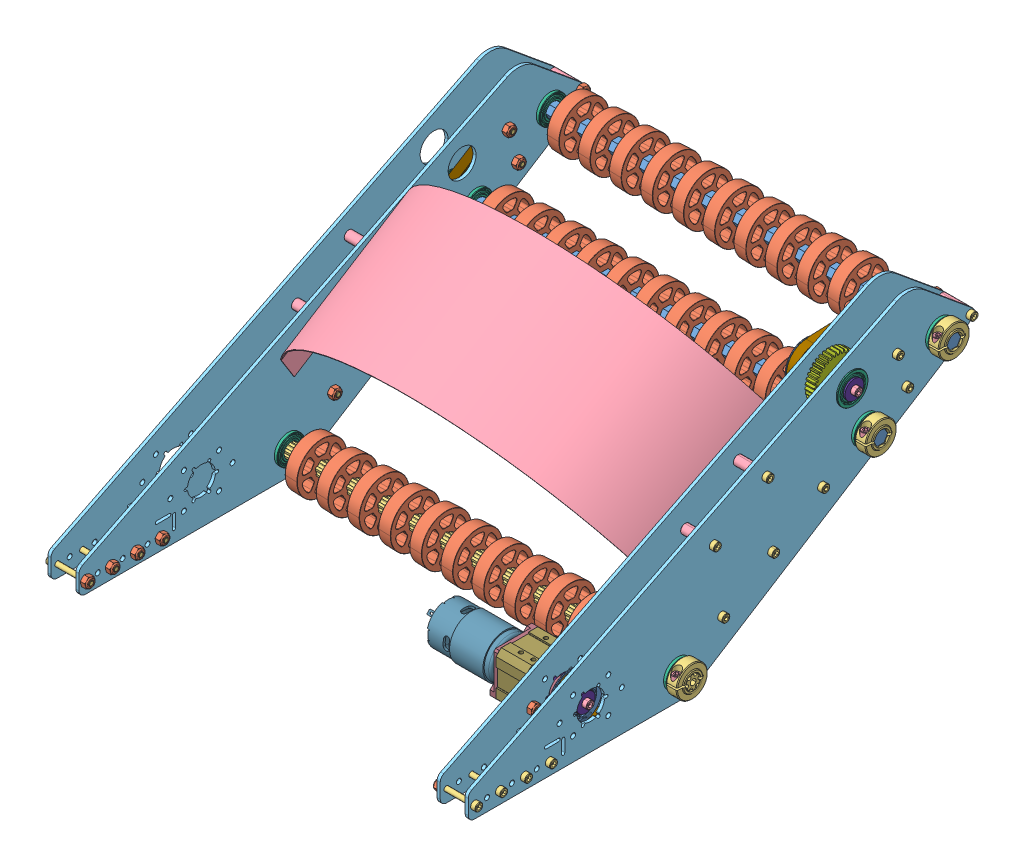
SolidWorks assembly am-4938 AndyMark Everybot Manipulator Assembly, configuration Default. Lengths in mm.
Overall size (460.38 280.97 519.68).
230 component instances, 40 part files, 0 mates.
Components (placement in the parent):
- am-4938 AndyMark Everybot Manipulator Assembly.STEP-1: am-4938 AndyMark Everybot Manipulator Assembly.STEP [Default] at origin size (460.38 280.97 519.68)
  - 9mm wide 24T 500 Hex.STEP-1: 9mm wide 24T 500 Hex.STEP [Default] at (375.9591 173.9174 489.4692) x (1 0 0) z (0 0.018419 0.99983) size (14 42 42)
    - am-3403 24 tooth HTD pulley half 500hex.STEP-1: am-3403 24 tooth HTD pulley half 500hex.STEP [Default] at (-136.5229 43.891 78.8344) size (8.91 42 42)
    - am-3403 24 tooth HTD pulley half 500hex.STEP-2: am-3403 24 tooth HTD pulley half 500hex.STEP [Default] at (-136.5229 43.891 36.8344) x (-1 0 0) z (0 0 -1) size (8.91 42 42)
  - 9mm wide 24T 500 Hex.STEP-2: 9mm wide 24T 500 Hex.STEP [Default] at (351.0194 381.3222 230.4036) x (1 0 0) z (0 -0.838389 0.545072) size (14 42 42)
    - am-3403 24 tooth HTD pulley half 500hex.STEP-1: am-3403 24 tooth HTD pulley half 500hex.STEP [Default] at (-136.5229 43.891 78.8344) size (8.91 42 42)
    - am-3403 24 tooth HTD pulley half 500hex.STEP-2: am-3403 24 tooth HTD pulley half 500hex.STEP [Default] at (-136.5229 43.891 36.8344) x (-1 0 0) z (0 0 -1) size (8.91 42 42)
  - 9mm wide 24T 500 Hex.STEP-3: 9mm wide 24T 500 Hex.STEP [Default] at (349.4573 384.489 140.1259) x (1 0 0) z (0 -0.834137 0.551557) size (14 42 42)
    - am-3403 24 tooth HTD pulley half 500hex.STEP-1: am-3403 24 tooth HTD pulley half 500hex.STEP [Default] at (-136.5229 43.891 78.8344) size (8.91 42 42)
    - am-3403 24 tooth HTD pulley half 500hex.STEP-2: am-3403 24 tooth HTD pulley half 500hex.STEP [Default] at (-136.5229 43.891 36.8344) x (-1 0 0) z (0 0 -1) size (8.91 42 42)
  - 9mm wide 24T 500 Hex.STEP-4: 9mm wide 24T 500 Hex.STEP [Default] at (375.9591 191.0878 396.7517) x (1 0 0) z (0 -0.5 0.866025) size (14 42 42)
    - am-3403 24 tooth HTD pulley half 500hex.STEP-1: am-3403 24 tooth HTD pulley half 500hex.STEP [Default] at (-136.5229 43.891 78.8344) size (8.91 42 42)
    - am-3403 24 tooth HTD pulley half 500hex.STEP-2: am-3403 24 tooth HTD pulley half 500hex.STEP [Default] at (-136.5229 43.891 36.8344) x (-1 0 0) z (0 0 -1) size (8.91 42 42)
  - AndyMark Everybot Spacer Subassembly.STEP-1: AndyMark Everybot Spacer Subassembly.STEP [Default] at (54.6794 -110.646 280.1551) size (42.93 11.21 11.21)
    - 10-32 Nylock Nut 1_90631A411.STEP-1: 10-32 Nylock Nut 1_90631A411.STEP [Default] at (168.4198 387.9509 141.8561) x (0 1 0) z (0 0 1) size (9.55 5.96 11.02)
    - 10-32x1500_shcs_HX-SHCS 0.19-32x1.375x1-C.STEP-1: 10-32x1500_shcs_HX-SHCS 0.19-32x1.375x1-C.STEP [Default] at (204.9958 387.9509 141.8561) x (-1 0 0) z (0 -0.673367 0.739309) size (42.93 7.94 7.94)
    - am-3876 1000long .192ID Aluminum Spacer.STEP-1: am-3876 1000long .192ID Aluminum Spacer.STEP [Default] at (171.5948 387.9509 141.8561) x (0 -0.090635 0.995884) z (0 0.995884 0.090635) size (9.53 25.4 9.53)
  - AndyMark Everybot Spacer Subassembly.STEP-2: AndyMark Everybot Spacer Subassembly.STEP [Default] at (54.6794 -37.8081 18.3964) size (42.93 11.21 11.21)
    - 10-32 Nylock Nut 1_90631A411.STEP-1: 10-32 Nylock Nut 1_90631A411.STEP [Default] at (168.4198 387.9509 141.8561) x (0 1 0) z (0 0 1) size (9.55 5.96 11.02)
    - 10-32x1500_shcs_HX-SHCS 0.19-32x1.375x1-C.STEP-1: 10-32x1500_shcs_HX-SHCS 0.19-32x1.375x1-C.STEP [Default] at (204.9958 387.9509 141.8561) x (-1 0 0) z (0 -0.673367 0.739309) size (42.93 7.94 7.94)
    - am-3876 1000long .192ID Aluminum Spacer.STEP-1: am-3876 1000long .192ID Aluminum Spacer.STEP [Default] at (171.5948 387.9509 141.8561) x (0 -0.090635 0.995884) z (0 0.995884 0.090635) size (9.53 25.4 9.53)
  - AndyMark Everybot Spacer Subassembly.STEP-3: AndyMark Everybot Spacer Subassembly.STEP [Default] at (54.6794 -76.9148 226.3549) size (42.93 11.21 11.21)
    - 10-32 Nylock Nut 1_90631A411.STEP-1: 10-32 Nylock Nut 1_90631A411.STEP [Default] at (168.4198 387.9509 141.8561) x (0 1 0) z (0 0 1) size (9.55 5.96 11.02)
    - 10-32x1500_shcs_HX-SHCS 0.19-32x1.375x1-C.STEP-1: 10-32x1500_shcs_HX-SHCS 0.19-32x1.375x1-C.STEP [Default] at (204.9958 387.9509 141.8561) x (-1 0 0) z (0 -0.673367 0.739309) size (42.93 7.94 7.94)
    - am-3876 1000long .192ID Aluminum Spacer.STEP-1: am-3876 1000long .192ID Aluminum Spacer.STEP [Default] at (171.5948 387.9509 141.8561) x (0 -0.090635 0.995884) z (0 0.995884 0.090635) size (9.53 25.4 9.53)
  - AndyMark Everybot Spacer Subassembly.STEP-4: AndyMark Everybot Spacer Subassembly.STEP [Default] at (54.6794 144.8465 -39.0656) x (1 0 0) z (0 -0.832151 0.55455) size (42.93 11.21 11.21)
    - 10-32 Nylock Nut 1_90631A411.STEP-1: 10-32 Nylock Nut 1_90631A411.STEP [Default] at (168.4198 387.9509 141.8561) x (0 1 0) z (0 0 1) size (9.55 5.96 11.02)
    - 10-32x1500_shcs_HX-SHCS 0.19-32x1.375x1-C.STEP-1: 10-32x1500_shcs_HX-SHCS 0.19-32x1.375x1-C.STEP [Default] at (204.9958 387.9509 141.8561) x (-1 0 0) z (0 -0.673367 0.739309) size (42.93 7.94 7.94)
    - am-3876 1000long .192ID Aluminum Spacer.STEP-1: am-3876 1000long .192ID Aluminum Spacer.STEP [Default] at (171.5948 387.9509 141.8561) x (0 -0.090635 0.995884) z (0 0.995884 0.090635) size (9.53 25.4 9.53)
  - 57 Sport 4_1 with Flange Mount and 775.STEP-1: 57 Sport 4_1 with Flange Mount and 775.STEP [Default] at (512.1422 191.8089 396.7872) size (148.8 62.86 82.55)
    - am-XXXX - 57 Sport 500 Hex Output Plug.STEP-1: am-XXXX - 57 Sport 500 Hex Output Plug.STEP [Default] at (-295.3931 6.0609 150.085) x (0 0 -1) z (1 0 0) size (44.45 44.45 56.57)
      - am-XXXX - 57 Sport 500 Hex Shaft.STEP-1: am-XXXX - 57 Sport 500 Hex Shaft.STEP [Default] at (0 0 6.1595) x (0.145042 0.989426 0) z (0 0 1) size (14.67 12.71 56.57)
      - Output Block.STEP-1: Output Block.STEP [Default] at origin size (44.45 44.45 20.32)
      - retaining Ring 0500 - Mcm 98410A122_98410A122.STEP-1: retaining Ring 0500 - Mcm 98410A122_98410A122.STEP [Default] at (0 0 -14.5034) x (0 0 1) z (-0.999848 0.017452 0) size (0.89 16.1 14.34)
      - R8ZZ Bearing.STEP-1: R8ZZ Bearing.STEP [Default] at (0 0 6.1595) x (0 0 -1) z (0.975423 0.220339 0) size (7.94 28.57 28.57)
      - R8ZZ Bearing.STEP-2: R8ZZ Bearing.STEP [Default] at (0 0 -5.842) x (0 0 -1) z (0.99707 -0.076493 0) size (7.94 28.57 28.57)
    - am-XXXX - 4_1 Input Stage.STEP-1: am-XXXX - 4_1 Input Stage.STEP [Default] at (-312.8556 6.0609 150.085) x (0 -0.369103 0.929389) z (-1 0 0) size (35.15 35.15 14.63)
      - am-XXXX - 57 Sport Shaft Carrier Plate.STEP-1: am-XXXX - 57 Sport Shaft Carrier Plate.STEP [Default] at origin size (31.12 31.12 14.63)
      - 16T Planet Gear.STEP-1: 16T Planet Gear.STEP [Default] at (-11.8222 1.3023 11.8494) x (0 0 -1) z (1 0 0) size (7.09 12.42 12.42)
      - 16T Planet Gear.STEP-2: 16T Planet Gear.STEP [Default] at (1.3023 11.8222 11.8494) x (0 0 -1) z (0 -1 0) size (7.09 12.42 12.42)
      - 16T Planet Gear.STEP-3: 16T Planet Gear.STEP [Default] at (11.8222 -1.3023 11.8494) x (0 0 -1) z (-1 0 0) size (7.09 12.42 12.42)
      - 16T Planet Gear.STEP-4: 16T Planet Gear.STEP [Default] at (-1.3023 -11.8222 11.8494) x (0 0 -1) z (0 1 0) size (7.09 12.42 12.42)
    - am-4132 57 Sport Flange Mount.STEP-1: am-4132 57 Sport Flange Mount.STEP [Default] at (-295.3931 6.0609 150.085) x (0 0 1) z (0 1 0) size (82.55 6.35 47.62)
    - am-XXXX - 57 Sport 1 Stage Ring Gear Housing.STEP-1: am-XXXX - 57 Sport 1 Stage Ring Gear Housing.STEP [Default] at (-314.3161 6.0609 150.085) x (0 -1 0) z (1 0 0) size (47.63 47.63 31.5)
    - am-3765 - 57 Sport Motor Block.STEP-1: am-3765 - 57 Sport Motor Block.STEP [Default] at (-333.8741 6.0609 150.085) x (0 0 -1) z (1 0 0) size (44.45 44.45 8.89)
    - 775 RedLine.STEP-1: 775 RedLine.STEP [Default] at (-337.6841 6.0609 150.085) x (-1 0 0) z (0 0.707107 -0.707107) size (87.75 44.83 44.07)
    - M4 x .7mm x 8mm SHCS_91290A140.STEP-1: M4 x .7mm x 8mm SHCS_91290A140.STEP [Default] at (-341.9503 -4.1921 139.8319) x (0 -0.977065 0.212941) z (-1 0 0) size (7 7 12.01)
    - M4 Lock Washer_91169A160.STEP-1: M4 Lock Washer_91169A160.STEP [Default] at (-333.1503 -4.1921 139.8319) x (0 0.294925 0.95552) z (-1 0 0) size (7.6 7.6 1.68)
    - M4 x .7mm x 8mm SHCS_91290A140.STEP-2: M4 x .7mm x 8mm SHCS_91290A140.STEP [Default] at (-341.9503 16.314 160.338) x (0 -0.411961 0.911202) z (-1 0 0) size (7 7 12.01)
    - M4 Lock Washer_91169A160.STEP-2: M4 Lock Washer_91169A160.STEP [Default] at (-333.0699 16.314 160.338) x (0 -0.95552 -0.294925) z (1 0 0) size (7.6 7.6 1.68)
    - am-3784 - RS-700 Motor Pinion Gear.STEP-1: am-3784 - RS-700 Motor Pinion Gear.STEP [Default] at (-323.5158 4.9342 148.4301) size (11.94 12.42 12.42)
    - 10-32 x 1.750 SHCS_90128A953.STEP-1: 10-32 x 1.750 SHCS_90128A953.STEP [Default] at (-339.8431 24.0214 132.1245) x (0 0.297258 -0.954797) z (-1 0 0) size (7.92 7.92 49.28)
    - 10-32 x 1.750 SHCS_90128A953.STEP-2: 10-32 x 1.750 SHCS_90128A953.STEP [Default] at (-339.8431 -11.8996 168.0455) x (0 -0.297258 0.954797) z (-1 0 0) size (7.92 7.92 49.28)
    - Thrust washer - 775 Sport.STEP-1: Thrust washer - 775 Sport.STEP [Default] at (-329.01 6.0609 150.085) x (0 0 -1) z (1 0 0) size (31 31 1.52)
    - BHCS 10-32 x 0.500_91255A265.STEP-1: BHCS 10-32 x 0.500_91255A265.STEP [Default] at (-289.6527 24.0214 168.0455) x (0 0 -1) z (1 0 0) size (9.17 9.17 15.27)
    - BHCS 10-32 x 0.500_91255A265.STEP-2: BHCS 10-32 x 0.500_91255A265.STEP [Default] at (-289.6527 -11.8996 132.1245) x (0 0 -1) z (1 0 0) size (9.17 9.17 15.27)
  - am-1526 500Hex Collar Clamp.STEP-1: am-1526 500Hex Collar Clamp.STEP [Default] at (238.9418 338.5749 286.0754) x (0 0.052851 0.998602) z (-1 0 0) size (31.72 31.75 12.7)
    - 500Hex Collar Clamp Body.STEP-1: 500Hex Collar Clamp Body.STEP [Default] at (-94.2794 15.3021 33.01) size (31.72 31.75 12.7)
    - 10-32x0500_shcs_HX-SHCS 0.19-32x1.375x1-C.STEP-1: 10-32x0500_shcs_HX-SHCS 0.19-32x1.375x1-C.STEP [Default] at (-83.1669 24.3191 39.36) x (0 -1 0) z (0 0 1) size (17.53 7.94 7.94)
  - am-1526 500Hex Collar Clamp.STEP-2: am-1526 500Hex Collar Clamp.STEP [Default] at (303.7214 290.7812 360.5945) x (0 0.052851 0.998602) z (-1 0 0) size (31.72 31.75 12.7)
    - 500Hex Collar Clamp Body.STEP-1: 500Hex Collar Clamp Body.STEP [Default] at (-94.2794 15.3021 33.01) size (31.72 31.75 12.7)
    - 10-32x0500_shcs_HX-SHCS 0.19-32x1.375x1-C.STEP-1: 10-32x0500_shcs_HX-SHCS 0.19-32x1.375x1-C.STEP [Default] at (-83.1669 24.3191 39.36) x (0 -1 0) z (0 0 1) size (17.53 7.94 7.94)
  - am-1526 500Hex Collar Clamp.STEP-3: am-1526 500Hex Collar Clamp.STEP [Default] at (303.7214 330.6759 284.8827) x (0 -0.030782 0.999526) z (-1 0 0) size (31.72 31.75 12.7)
    - 500Hex Collar Clamp Body.STEP-1: 500Hex Collar Clamp Body.STEP [Default] at (-94.2794 15.3021 33.01) size (31.72 31.75 12.7)
    - 10-32x0500_shcs_HX-SHCS 0.19-32x1.375x1-C.STEP-1: 10-32x0500_shcs_HX-SHCS 0.19-32x1.375x1-C.STEP [Default] at (-83.1669 24.3191 39.36) x (0 -1 0) z (0 0 1) size (17.53 7.94 7.94)
  - am-1526 500Hex Collar Clamp.STEP-4: am-1526 500Hex Collar Clamp.STEP [Default] at (303.7214 171.6969 553.2396) x (0 0.052851 0.998602) z (-1 0 0) size (31.72 31.75 12.7)
    - 500Hex Collar Clamp Body.STEP-1: 500Hex Collar Clamp Body.STEP [Default] at (-94.2794 15.3021 33.01) size (31.72 31.75 12.7)
    - 10-32x0500_shcs_HX-SHCS 0.19-32x1.375x1-C.STEP-1: 10-32x0500_shcs_HX-SHCS 0.19-32x1.375x1-C.STEP [Default] at (-83.1669 24.3191 39.36) x (0 -1 0) z (0 0 1) size (17.53 7.94 7.94)
  - AndyMark Everybot Spacer Subassembly.STEP-5: AndyMark Everybot Spacer Subassembly.STEP [Default] at (26.3939 261.0166 834.7627) x (-1 0 0) z (0 -0.924911 -0.380184) size (42.93 11.21 11.21)
    - 10-32 Nylock Nut 1_90631A411.STEP-1: 10-32 Nylock Nut 1_90631A411.STEP [Default] at (168.4198 387.9509 141.8561) x (0 1 0) z (0 0 1) size (9.55 5.96 11.02)
    - 10-32x1500_shcs_HX-SHCS 0.19-32x1.375x1-C.STEP-1: 10-32x1500_shcs_HX-SHCS 0.19-32x1.375x1-C.STEP [Default] at (204.9958 387.9509 141.8561) x (-1 0 0) z (0 -0.673367 0.739309) size (42.93 7.94 7.94)
    - am-3876 1000long .192ID Aluminum Spacer.STEP-1: am-3876 1000long .192ID Aluminum Spacer.STEP [Default] at (171.5948 387.9509 141.8561) x (0 -0.090635 0.995884) z (0 0.995884 0.090635) size (9.53 25.4 9.53)
  - AndyMark Everybot Spacer Subassembly.STEP-6: AndyMark Everybot Spacer Subassembly.STEP [Default] at (26.3939 294.7478 780.9625) x (-1 0 0) z (0 -0.924911 -0.380184) size (42.93 11.21 11.21)
    - 10-32 Nylock Nut 1_90631A411.STEP-1: 10-32 Nylock Nut 1_90631A411.STEP [Default] at (168.4198 387.9509 141.8561) x (0 1 0) z (0 0 1) size (9.55 5.96 11.02)
    - 10-32x1500_shcs_HX-SHCS 0.19-32x1.375x1-C.STEP-1: 10-32x1500_shcs_HX-SHCS 0.19-32x1.375x1-C.STEP [Default] at (204.9958 387.9509 141.8561) x (-1 0 0) z (0 -0.673367 0.739309) size (42.93 7.94 7.94)
    - am-3876 1000long .192ID Aluminum Spacer.STEP-1: am-3876 1000long .192ID Aluminum Spacer.STEP [Default] at (171.5948 387.9509 141.8561) x (0 -0.090635 0.995884) z (0 0.995884 0.090635) size (9.53 25.4 9.53)
  - AndyMark Everybot Spacer Subassembly.STEP-7: AndyMark Everybot Spacer Subassembly.STEP [Default] at (26.3939 225.6505 775.1858) x (-1 0 0) z (0 -0.924911 -0.380184) size (42.93 11.21 11.21)
    - 10-32 Nylock Nut 1_90631A411.STEP-1: 10-32 Nylock Nut 1_90631A411.STEP [Default] at (168.4198 387.9509 141.8561) x (0 1 0) z (0 0 1) size (9.55 5.96 11.02)
    - 10-32x1500_shcs_HX-SHCS 0.19-32x1.375x1-C.STEP-1: 10-32x1500_shcs_HX-SHCS 0.19-32x1.375x1-C.STEP [Default] at (204.9958 387.9509 141.8561) x (-1 0 0) z (0 -0.673367 0.739309) size (42.93 7.94 7.94)
    - am-3876 1000long .192ID Aluminum Spacer.STEP-1: am-3876 1000long .192ID Aluminum Spacer.STEP [Default] at (171.5948 387.9509 141.8561) x (0 -0.090635 0.995884) z (0 0.995884 0.090635) size (9.53 25.4 9.53)
  - AndyMark Everybot Spacer Subassembly.STEP-8: AndyMark Everybot Spacer Subassembly.STEP [Default] at (26.3939 333.8545 573.004) x (-1 0 0) z (0 -0.924911 -0.380184) size (42.93 11.21 11.21)
    - 10-32 Nylock Nut 1_90631A411.STEP-1: 10-32 Nylock Nut 1_90631A411.STEP [Default] at (168.4198 387.9509 141.8561) x (0 1 0) z (0 0 1) size (9.55 5.96 11.02)
    - 10-32x1500_shcs_HX-SHCS 0.19-32x1.375x1-C.STEP-1: 10-32x1500_shcs_HX-SHCS 0.19-32x1.375x1-C.STEP [Default] at (204.9958 387.9509 141.8561) x (-1 0 0) z (0 -0.673367 0.739309) size (42.93 7.94 7.94)
    - am-3876 1000long .192ID Aluminum Spacer.STEP-1: am-3876 1000long .192ID Aluminum Spacer.STEP [Default] at (171.5948 387.9509 141.8561) x (0 -0.090635 0.995884) z (0 0.995884 0.090635) size (9.53 25.4 9.53)
  - am-1526 500Hex Collar Clamp.STEP-5: am-1526 500Hex Collar Clamp.STEP [Default] at (-143.9282 338.5749 286.0754) x (0 0.052851 0.998602) z (-1 0 0) size (31.72 31.75 12.7)
    - 500Hex Collar Clamp Body.STEP-1: 500Hex Collar Clamp Body.STEP [Default] at (-94.2794 15.3021 33.01) size (31.72 31.75 12.7)
    - 10-32x0500_shcs_HX-SHCS 0.19-32x1.375x1-C.STEP-1: 10-32x0500_shcs_HX-SHCS 0.19-32x1.375x1-C.STEP [Default] at (-83.1669 24.3191 39.36) x (0 -1 0) z (0 0 1) size (17.53 7.94 7.94)
  - am-1526 500Hex Collar Clamp.STEP-6: am-1526 500Hex Collar Clamp.STEP [Default] at (-143.9282 291.5849 361.5416) x (0 0.052851 0.998602) z (-1 0 0) size (31.72 31.75 12.7)
    - 500Hex Collar Clamp Body.STEP-1: 500Hex Collar Clamp Body.STEP [Default] at (-94.2794 15.3021 33.01) size (31.72 31.75 12.7)
    - 10-32x0500_shcs_HX-SHCS 0.19-32x1.375x1-C.STEP-1: 10-32x0500_shcs_HX-SHCS 0.19-32x1.375x1-C.STEP [Default] at (-83.1669 24.3191 39.36) x (0 -1 0) z (0 0 1) size (17.53 7.94 7.94)
  - am-1526 500Hex Collar Clamp.STEP-7: am-1526 500Hex Collar Clamp.STEP [Default] at (-143.9282 171.6969 553.2396) x (0 0.052851 0.998602) z (-1 0 0) size (31.72 31.75 12.7)
    - 500Hex Collar Clamp Body.STEP-1: 500Hex Collar Clamp Body.STEP [Default] at (-94.2794 15.3021 33.01) size (31.72 31.75 12.7)
    - 10-32x0500_shcs_HX-SHCS 0.19-32x1.375x1-C.STEP-1: 10-32x0500_shcs_HX-SHCS 0.19-32x1.375x1-C.STEP [Default] at (-83.1669 24.3191 39.36) x (0 -1 0) z (0 0 1) size (17.53 7.94 7.94)
  - 9mm wide 24T 500 Hex.STEP-5: 9mm wide 24T 500 Hex.STEP [Default] at (-22.0558 172.1698 396.8644) x (1 0 0) z (0 -0.216531 0.976276) size (14 42 42)
    - am-3403 24 tooth HTD pulley half 500hex.STEP-1: am-3403 24 tooth HTD pulley half 500hex.STEP [Default] at (-136.5229 43.891 78.8344) size (8.91 42 42)
    - am-3403 24 tooth HTD pulley half 500hex.STEP-2: am-3403 24 tooth HTD pulley half 500hex.STEP [Default] at (-136.5229 43.891 36.8344) x (-1 0 0) z (0 0 -1) size (8.91 42 42)
  - 9mm wide 24T 500 Hex.STEP-6: 9mm wide 24T 500 Hex.STEP [Default] at (-22.0558 323.6557 134.2603) x (1 0 0) z (0 0.040546 0.999178) size (14 42 42)
    - am-3403 24 tooth HTD pulley half 500hex.STEP-1: am-3403 24 tooth HTD pulley half 500hex.STEP [Default] at (-136.5229 43.891 78.8344) size (8.91 42 42)
    - am-3403 24 tooth HTD pulley half 500hex.STEP-2: am-3403 24 tooth HTD pulley half 500hex.STEP [Default] at (-136.5229 43.891 36.8344) x (-1 0 0) z (0 0 -1) size (8.91 42 42)
  - AndyMark Everybot Spacer Subassembly.STEP-9: AndyMark Everybot Spacer Subassembly.STEP [Default] at (26.3939 336.767 648.1233) x (-1 0 0) z (0 -0.924911 -0.380184) size (42.93 11.21 11.21)
    - 10-32 Nylock Nut 1_90631A411.STEP-1: 10-32 Nylock Nut 1_90631A411.STEP [Default] at (168.4198 387.9509 141.8561) x (0 1 0) z (0 0 1) size (9.55 5.96 11.02)
    - 10-32x1500_shcs_HX-SHCS 0.19-32x1.375x1-C.STEP-1: 10-32x1500_shcs_HX-SHCS 0.19-32x1.375x1-C.STEP [Default] at (204.9958 387.9509 141.8561) x (-1 0 0) z (0 -0.673367 0.739309) size (42.93 7.94 7.94)
    - am-3876 1000long .192ID Aluminum Spacer.STEP-1: am-3876 1000long .192ID Aluminum Spacer.STEP [Default] at (171.5948 387.9509 141.8561) x (0 -0.090635 0.995884) z (0 0.995884 0.090635) size (9.53 25.4 9.53)
  - AndyMark Everybot Spacer Subassembly.STEP-10: AndyMark Everybot Spacer Subassembly.STEP [Default] at (26.3939 303.189 638.5172) x (-1 0 0) z (0 -0.924911 -0.380184) size (42.93 11.21 11.21)
    - 10-32 Nylock Nut 1_90631A411.STEP-1: 10-32 Nylock Nut 1_90631A411.STEP [Default] at (168.4198 387.9509 141.8561) x (0 1 0) z (0 0 1) size (9.55 5.96 11.02)
    - 10-32x1500_shcs_HX-SHCS 0.19-32x1.375x1-C.STEP-1: 10-32x1500_shcs_HX-SHCS 0.19-32x1.375x1-C.STEP [Default] at (204.9958 387.9509 141.8561) x (-1 0 0) z (0 -0.673367 0.739309) size (42.93 7.94 7.94)
    - am-3876 1000long .192ID Aluminum Spacer.STEP-1: am-3876 1000long .192ID Aluminum Spacer.STEP [Default] at (171.5948 387.9509 141.8561) x (0 -0.090635 0.995884) z (0 0.995884 0.090635) size (9.53 25.4 9.53)
  - AndyMark Everybot Spacer Subassembly.STEP-11: AndyMark Everybot Spacer Subassembly.STEP [Default] at (26.3939 256.8115 724.2868) x (-1 0 0) z (0 -0.924307 -0.38165) size (42.93 11.21 11.21)
    - 10-32 Nylock Nut 1_90631A411.STEP-1: 10-32 Nylock Nut 1_90631A411.STEP [Default] at (168.4198 387.9509 141.8561) x (0 1 0) z (0 0 1) size (9.55 5.96 11.02)
    - 10-32x1500_shcs_HX-SHCS 0.19-32x1.375x1-C.STEP-1: 10-32x1500_shcs_HX-SHCS 0.19-32x1.375x1-C.STEP [Default] at (204.9958 387.9509 141.8561) x (-1 0 0) z (0 -0.673367 0.739309) size (42.93 7.94 7.94)
    - am-3876 1000long .192ID Aluminum Spacer.STEP-1: am-3876 1000long .192ID Aluminum Spacer.STEP [Default] at (171.5948 387.9509 141.8561) x (0 -0.090635 0.995884) z (0 0.995884 0.090635) size (9.53 25.4 9.53)
  - AndyMark Everybot Spacer Subassembly.STEP-12: AndyMark Everybot Spacer Subassembly.STEP [Default] at (26.3939 193.7876 826.1337) x (-1 0 0) z (0 -0.924911 -0.380184) size (42.93 11.21 11.21)
    - 10-32 Nylock Nut 1_90631A411.STEP-1: 10-32 Nylock Nut 1_90631A411.STEP [Default] at (168.4198 387.9509 141.8561) x (0 1 0) z (0 0 1) size (9.55 5.96 11.02)
    - 10-32x1500_shcs_HX-SHCS 0.19-32x1.375x1-C.STEP-1: 10-32x1500_shcs_HX-SHCS 0.19-32x1.375x1-C.STEP [Default] at (204.9958 387.9509 141.8561) x (-1 0 0) z (0 -0.673367 0.739309) size (42.93 7.94 7.94)
    - am-3876 1000long .192ID Aluminum Spacer.STEP-1: am-3876 1000long .192ID Aluminum Spacer.STEP [Default] at (171.5948 387.9509 141.8561) x (0 -0.090635 0.995884) z (0 0.995884 0.090635) size (9.53 25.4 9.53)
  - AndyMark Everybot Spacer Subassembly.STEP-13: AndyMark Everybot Spacer Subassembly.STEP [Default] at (54.6794 509.1158 698.3459) x (1 0 0) z (0 0.399295 -0.916823) size (42.93 11.21 11.21)
    - 10-32 Nylock Nut 1_90631A411.STEP-1: 10-32 Nylock Nut 1_90631A411.STEP [Default] at (168.4198 387.9509 141.8561) x (0 1 0) z (0 0 1) size (9.55 5.96 11.02)
    - 10-32x1500_shcs_HX-SHCS 0.19-32x1.375x1-C.STEP-1: 10-32x1500_shcs_HX-SHCS 0.19-32x1.375x1-C.STEP [Default] at (204.9958 387.9509 141.8561) x (-1 0 0) z (0 -0.673367 0.739309) size (42.93 7.94 7.94)
    - am-3876 1000long .192ID Aluminum Spacer.STEP-1: am-3876 1000long .192ID Aluminum Spacer.STEP [Default] at (171.5948 387.9509 141.8561) x (0 -0.090635 0.995884) z (0 0.995884 0.090635) size (9.53 25.4 9.53)
  - AndyMark Everybot Spacer Subassembly.STEP-14: AndyMark Everybot Spacer Subassembly.STEP [Default] at (54.6794 618.5172 510.7294) x (1 0 0) z (0 0.399295 -0.916823) size (42.93 11.21 11.21)
    - 10-32 Nylock Nut 1_90631A411.STEP-1: 10-32 Nylock Nut 1_90631A411.STEP [Default] at (168.4198 387.9509 141.8561) x (0 1 0) z (0 0 1) size (9.55 5.96 11.02)
    - 10-32x1500_shcs_HX-SHCS 0.19-32x1.375x1-C.STEP-1: 10-32x1500_shcs_HX-SHCS 0.19-32x1.375x1-C.STEP [Default] at (204.9958 387.9509 141.8561) x (-1 0 0) z (0 -0.673367 0.739309) size (42.93 7.94 7.94)
    - am-3876 1000long .192ID Aluminum Spacer.STEP-1: am-3876 1000long .192ID Aluminum Spacer.STEP [Default] at (171.5948 387.9509 141.8561) x (0 -0.090635 0.995884) z (0 0.995884 0.090635) size (9.53 25.4 9.53)
  - AndyMark Everybot Spacer Subassembly.STEP-15: AndyMark Everybot Spacer Subassembly.STEP [Default] at (54.6794 572.7943 596.5254) x (1 0 0) z (0 0.399295 -0.916823) size (42.93 11.21 11.21)
    - 10-32 Nylock Nut 1_90631A411.STEP-1: 10-32 Nylock Nut 1_90631A411.STEP [Default] at (168.4198 387.9509 141.8561) x (0 1 0) z (0 0 1) size (9.55 5.96 11.02)
    - 10-32x1500_shcs_HX-SHCS 0.19-32x1.375x1-C.STEP-1: 10-32x1500_shcs_HX-SHCS 0.19-32x1.375x1-C.STEP [Default] at (204.9958 387.9509 141.8561) x (-1 0 0) z (0 -0.673367 0.739309) size (42.93 7.94 7.94)
    - am-3876 1000long .192ID Aluminum Spacer.STEP-1: am-3876 1000long .192ID Aluminum Spacer.STEP [Default] at (171.5948 387.9509 141.8561) x (0 -0.090635 0.995884) z (0 0.995884 0.090635) size (9.53 25.4 9.53)
  - AndyMark Everybot Spacer Subassembly.STEP-16: AndyMark Everybot Spacer Subassembly.STEP [Default] at (54.6794 652.0951 520.3355) x (1 0 0) z (0 0.399295 -0.916823) size (42.93 11.21 11.21)
    - 10-32 Nylock Nut 1_90631A411.STEP-1: 10-32 Nylock Nut 1_90631A411.STEP [Default] at (168.4198 387.9509 141.8561) x (0 1 0) z (0 0 1) size (9.55 5.96 11.02)
    - 10-32x1500_shcs_HX-SHCS 0.19-32x1.375x1-C.STEP-1: 10-32x1500_shcs_HX-SHCS 0.19-32x1.375x1-C.STEP [Default] at (204.9958 387.9509 141.8561) x (-1 0 0) z (0 -0.673367 0.739309) size (42.93 7.94 7.94)
    - am-3876 1000long .192ID Aluminum Spacer.STEP-1: am-3876 1000long .192ID Aluminum Spacer.STEP [Default] at (171.5948 387.9509 141.8561) x (0 -0.090635 0.995884) z (0 0.995884 0.090635) size (9.53 25.4 9.53)
  - am-4938_in-plate AndyMark EveryBot Intake Plate_V2.STEP-1: am-4938_in-plate AndyMark EveryBot Intake Plate_V2.STEP [Default] at (254.8492 156.5948 671.6871) size (3.17 244.43 516.2)
  - am-4938_in-plate AndyMark EveryBot Intake Plate_V2.STEP-2: am-4938_in-plate AndyMark EveryBot Intake Plate_V2.STEP [Default] at (226.2742 156.5948 671.6871) size (3.17 244.43 516.2)
  - am-2986 FR8ZZ Hex Bearing.STEP-1: am-2986 FR8ZZ Hex Bearing.STEP [Default] at (256.4494 345.3116 281.1191) x (0 -0.052851 -0.998602) z (0 -0.998602 0.052851) size (31.12 7.94 31.12)
  - am-2986 FR8ZZ Hex Bearing.STEP-2: am-2986 FR8ZZ Hex Bearing.STEP [Default] at (221.499 345.3116 281.1191) x (0 0.838389 -0.545072) z (0 0.545072 0.838389) size (31.12 7.94 31.12)
  - am-4709 36T 20DP 500hex 375 FW.STEP-1: am-4709 36T 20DP 500hex 375 FW.STEP [Default] at (231.024 345.3116 281.1191) x (1 0 0) z (0 0.891241 0.453531) size (12.7 48.15 48.15)
  - am-3948-250 500H x 250IN Spacer.STEP-1: am-3948-250 500H x 250IN Spacer.STEP [Default] at (248.4865 345.3116 281.1191) x (0 0.052851 0.998602) z (-1 0 0) size (20 20 6.35)
  - am-4902 60T 5mm HTD Belt 9mm Wide.STEP-1: am-4902 60T 5mm HTD Belt 9mm Wide.STEP [Default] at (208.9344 345.3144 281.0487) x (1 0 0) z (0 -0.039538 0.999218) size (9 41.68 131.68)
  - am-4902 60T 5mm HTD Belt 9mm Wide.STEP-2: am-4902 60T 5mm HTD Belt 9mm Wide.STEP [Default] at (235.4362 197.8698 546.8722) x (1 0 0) z (0 0.176389 0.984321) size (9 41.68 131.68)
  - am-1692 2 in. Long 0.5 in OD F-F Steel Standoff_92230A135.STEP-1: am-1692 2 in. Long 0.5 in OD F-F Steel Standoff_92230A135.STEP [Default] at (231.0494 345.3116 281.1191) x (0 -0.453531 0.891241) z (1 0 0) size (14.71 14.77 59.16)
  - am-3948-063 500H x 063IN Spacer.STEP-1: am-3948-063 500H x 063IN Spacer.STEP [Default] at (206.0278 345.3116 281.1191) x (0 0.891241 0.453531) z (1 0 0) size (20 20 1.59)
  - 10-32x0500_shcs_HX-SHCS 0.19-32x1.375x1-C.STEP-1: 10-32x0500_shcs_HX-SHCS 0.19-32x1.375x1-C.STEP [Default] at (199.6143 345.3116 281.1191) x (1 0 0) z (0 0.014609 0.999893) size (17.53 7.94 7.94)
  - 10-32 Nylock Nut 1_90631A411.STEP-1: 10-32 Nylock Nut 1_90631A411.STEP [Default] at (226.2742 197.8698 515.1222) x (0 0.902435 0.430825) z (0 0.430825 -0.902435) size (9.55 5.96 11.02)
  - 10-32 Nylock Nut 1_90631A411.STEP-2: 10-32 Nylock Nut 1_90631A411.STEP [Default] at (226.2742 197.8698 578.6222) x (0 0.845049 0.534689) z (0 0.534689 -0.845049) size (9.55 5.96 11.02)
  - 10-32x750_shcs_90128A945.STEP-1: 10-32x750_shcs_90128A945.STEP [Default] at (235.7992 197.8698 515.1222) x (0 -0.644782 -0.764367) z (1 0 0) size (7.92 7.92 23.88)
  - 10-32x750_shcs_90128A945.STEP-2: 10-32x750_shcs_90128A945.STEP [Default] at (235.7992 197.8698 578.6222) x (0 0 -1) z (1 0 0) size (7.92 7.92 23.88)
  - am-3948-375 500H x 375IN Spacer.STEP-1: am-3948-375 500H x 375IN Spacer.STEP [Default] at (232.4337 197.8698 546.8722) x (0 0.091272 -0.995826) z (-1 0 0) size (20 20 9.53)
  - am-3948-063 500H x 063IN Spacer.STEP-2: am-3948-063 500H x 063IN Spacer.STEP [Default] at (248.0261 197.8698 546.8722) x (0 0.620323 0.784347) z (-1 0 0) size (20 20 1.59)
  - am-2986 FR8ZZ Hex Bearing.STEP-3: am-2986 FR8ZZ Hex Bearing.STEP [Default] at (227.8744 348.8728 191.1191) x (0 -0.052851 -0.998602) z (0 -0.998602 0.052851) size (31.12 7.94 31.12)
  - am-2986 FR8ZZ Hex Bearing.STEP-4: am-2986 FR8ZZ Hex Bearing.STEP [Default] at (250.074 348.8728 191.1191) x (0 0.902752 0.430162) z (0 -0.430162 0.902752) size (31.12 7.94 31.12)
  - am-3948-375 500H x 375IN Spacer.STEP-2: am-3948-375 500H x 375IN Spacer.STEP [Default] at (227.849 348.8728 191.1191) x (0 0.091272 0.995826) z (1 0 0) size (20 20 9.53)
  - am-3948-375 500H x 375IN Spacer.STEP-3: am-3948-375 500H x 375IN Spacer.STEP [Default] at (250.0994 301.8828 266.5853) x (0 0.091272 -0.995826) z (-1 0 0) size (20 20 9.53)
  - am-4709 36T 20DP 500hex 375 FW.STEP-2: am-4709 36T 20DP 500hex 375 FW.STEP [Default] at (229.4619 301.8828 266.5853) x (1 0 0) z (0 0.813642 0.581366) size (12.7 48.15 48.15)
  - am-2986 FR8ZZ Hex Bearing.STEP-5: am-2986 FR8ZZ Hex Bearing.STEP [Default] at (250.074 301.8828 266.5853) x (0 0.902752 0.430162) z (0 -0.430162 0.902752) size (31.12 7.94 31.12)
  - am-2986 FR8ZZ Hex Bearing.STEP-6: am-2986 FR8ZZ Hex Bearing.STEP [Default] at (227.8744 301.8828 266.5853) x (0 -0.052851 -0.998602) z (0 -0.998602 0.052851) size (31.12 7.94 31.12)
  - am-3948-500 500H x 500IN Spacer.STEP-1: am-3948-500 500H x 500IN Spacer.STEP [Default] at (250.074 348.8728 191.1191) x (0 0 1) z (-1 0 0) size (20 20 12.7)
  - am-2986 FR8ZZ Hex Bearing.STEP-7: am-2986 FR8ZZ Hex Bearing.STEP [Default] at (250.074 181.9948 458.2833) x (0 1 0) z (0 0 1) size (31.12 7.94 31.12)
  - am-2986 FR8ZZ Hex Bearing.STEP-8: am-2986 FR8ZZ Hex Bearing.STEP [Default] at (227.8744 181.9948 458.2833) x (0 0.381849 -0.924225) z (0 -0.924225 -0.381849) size (31.12 7.94 31.12)
  - am-3948-188 500H x 188IN Spacer.STEP-1: am-3948-188 500H x 188IN Spacer.STEP [Default] at (227.8744 181.9948 458.2833) x (0 -0.039215 -0.999231) z (1 0 0) size (20 20 4.78)
  - am-3948-125 500H x 125IN Spacer.STEP-1: am-3948-125 500H x 125IN Spacer.STEP [Default] at (246.899 181.9948 458.2833) x (0 -0.062923 0.998018) z (1 0 0) size (20 20 3.17)
  - am-1523 10 Fender Washer.STEP-1: am-1523 10 Fender Washer.STEP [Default] at (204.4403 345.3116 281.1191) x (0 -1 0) z (0 0 1) size (19.05 1.59 19.05)
  - am-1523 10 Fender Washer.STEP-2: am-1523 10 Fender Washer.STEP [Default] at (256.4494 345.3116 281.1191) x (0 -0.381849 0.924225) z (0 0.924225 0.381849) size (19.05 1.59 19.05)
  - 10-32x0500_shcs_HX-SHCS 0.19-32x1.375x1-C.STEP-2: 10-32x0500_shcs_HX-SHCS 0.19-32x1.375x1-C.STEP [Default] at (262.8629 345.3116 281.1191) x (-1 0 0) z (0 -0.924225 -0.381849) size (17.53 7.94 7.94)
  - am-1523 10 Fender Washer.STEP-3: am-1523 10 Fender Washer.STEP [Default] at (248.3087 197.8698 546.8722) x (0 -0.381849 0.924225) z (0 0.924225 0.381849) size (19.05 1.59 19.05)
  - 10-32x0500_shcs_HX-SHCS 0.19-32x1.375x1-C.STEP-3: 10-32x0500_shcs_HX-SHCS 0.19-32x1.375x1-C.STEP [Default] at (254.7222 197.8698 546.8722) x (-1 0 0) z (0 -0.924225 -0.381849) size (17.53 7.94 7.94)
  - 10-32x1500_shcs_HX-SHCS 0.19-32x1.375x1-C.STEP-1: 10-32x1500_shcs_HX-SHCS 0.19-32x1.375x1-C.STEP [Default] at (259.6752 169.2948 589.1371) x (-1 0 0) z (0 -0.673367 0.739309) size (42.93 7.94 7.94)
  - 10-32x1500_shcs_HX-SHCS 0.19-32x1.375x1-C.STEP-2: 10-32x1500_shcs_HX-SHCS 0.19-32x1.375x1-C.STEP [Default] at (259.6752 169.2948 614.5371) x (-1 0 0) z (0 -0.673367 0.739309) size (42.93 7.94 7.94)
  - 10-32x1500_shcs_HX-SHCS 0.19-32x1.375x1-C.STEP-3: 10-32x1500_shcs_HX-SHCS 0.19-32x1.375x1-C.STEP [Default] at (259.6752 169.2948 639.9371) x (-1 0 0) z (0 -0.673367 0.739309) size (42.93 7.94 7.94)
  - 10-32x1500_shcs_HX-SHCS 0.19-32x1.375x1-C.STEP-4: 10-32x1500_shcs_HX-SHCS 0.19-32x1.375x1-C.STEP [Default] at (259.6752 169.2948 665.3371) x (-1 0 0) z (0 -0.673367 0.739309) size (42.93 7.94 7.94)
  - 10-32 Nylock Nut 1_90631A411.STEP-3: 10-32 Nylock Nut 1_90631A411.STEP [Default] at (223.0992 169.2948 589.1371) x (0 0.488303 0.872674) z (0 -0.872674 0.488303) size (9.55 5.96 11.02)
  - 10-32 Nylock Nut 1_90631A411.STEP-4: 10-32 Nylock Nut 1_90631A411.STEP [Default] at (223.0992 169.2948 614.5371) x (0 0.488303 0.872674) z (0 -0.872674 0.488303) size (9.55 5.96 11.02)
  - 10-32 Nylock Nut 1_90631A411.STEP-5: 10-32 Nylock Nut 1_90631A411.STEP [Default] at (223.0992 169.2948 639.9371) x (0 0.488303 0.872674) z (0 -0.872674 0.488303) size (9.55 5.96 11.02)
  - 10-32 Nylock Nut 1_90631A411.STEP-6: 10-32 Nylock Nut 1_90631A411.STEP [Default] at (223.0992 169.2948 665.3371) x (0 0.488303 0.872674) z (0 -0.872674 0.488303) size (9.55 5.96 11.02)
  - am-4938_in-plate AndyMark EveryBot Intake Plate_V2.STEP-3: am-4938_in-plate AndyMark EveryBot Intake Plate_V2.STEP [Default] at (-142.0258 156.5948 671.6871) size (3.17 244.43 516.2)
  - am-4938_in-plate AndyMark EveryBot Intake Plate_V2.STEP-4: am-4938_in-plate AndyMark EveryBot Intake Plate_V2.STEP [Default] at (-170.6008 156.5948 671.6871) size (3.17 244.43 516.2)
  - 10-32x1500_shcs_HX-SHCS 0.19-32x1.375x1-C.STEP-5: 10-32x1500_shcs_HX-SHCS 0.19-32x1.375x1-C.STEP [Default] at (-178.6018 169.2948 665.3371) x (1 0 0) z (0 0.940412 -0.340038) size (42.93 7.94 7.94)
  - 10-32x1500_shcs_HX-SHCS 0.19-32x1.375x1-C.STEP-6: 10-32x1500_shcs_HX-SHCS 0.19-32x1.375x1-C.STEP [Default] at (-178.6018 169.2948 639.9371) x (1 0 0) z (0 0.940412 -0.340038) size (42.93 7.94 7.94)
  - 10-32x1500_shcs_HX-SHCS 0.19-32x1.375x1-C.STEP-7: 10-32x1500_shcs_HX-SHCS 0.19-32x1.375x1-C.STEP [Default] at (-178.6018 169.2948 614.5371) x (1 0 0) z (0 0.940412 -0.340038) size (42.93 7.94 7.94)
  - 10-32x1500_shcs_HX-SHCS 0.19-32x1.375x1-C.STEP-8: 10-32x1500_shcs_HX-SHCS 0.19-32x1.375x1-C.STEP [Default] at (-178.6018 169.2948 589.1371) x (1 0 0) z (0 0.940412 -0.340038) size (42.93 7.94 7.94)
  - am-2986 FR8ZZ Hex Bearing.STEP-9: am-2986 FR8ZZ Hex Bearing.STEP [Default] at (-146.801 348.8728 191.1191) x (0 0.902752 0.430162) z (0 -0.430162 0.902752) size (31.12 7.94 31.12)
  - am-2986 FR8ZZ Hex Bearing.STEP-10: am-2986 FR8ZZ Hex Bearing.STEP [Default] at (-169.0006 348.8728 191.1191) x (0 -0.052851 -0.998602) z (0 -0.998602 0.052851) size (31.12 7.94 31.12)
  - am-2986 FR8ZZ Hex Bearing.STEP-11: am-2986 FR8ZZ Hex Bearing.STEP [Default] at (-146.801 301.8828 266.5853) x (0 0.902752 0.430162) z (0 -0.430162 0.902752) size (31.12 7.94 31.12)
  - am-2986 FR8ZZ Hex Bearing.STEP-12: am-2986 FR8ZZ Hex Bearing.STEP [Default] at (-169.0006 301.8828 266.5853) x (0 -0.052851 -0.998602) z (0 -0.998602 0.052851) size (31.12 7.94 31.12)
  - am-2986 FR8ZZ Hex Bearing.STEP-13: am-2986 FR8ZZ Hex Bearing.STEP [Default] at (-146.801 181.9948 458.2833) x (0 0.887213 0.46136) z (0 -0.46136 0.887213) size (31.12 7.94 31.12)
  - am-2986 FR8ZZ Hex Bearing.STEP-14: am-2986 FR8ZZ Hex Bearing.STEP [Default] at (-169.0006 181.9948 458.2833) x (0 -0.052851 -0.998602) z (0 -0.998602 0.052851) size (31.12 7.94 31.12)
  - am-4911 150T 5mm HTD Belt 9mm Wide.STEP-1: am-4911 150T 5mm HTD Belt 9mm Wide.STEP [Default] at (-162.5787 181.9948 458.2833) x (1 0 0) z (0 -0.529771 0.84814) size (9 41.68 356.68)
  - am-3948-188 500H x 188IN Spacer.STEP-2: am-3948-188 500H x 188IN Spacer.STEP [Default] at (-151.5762 181.9948 458.2833) x (0 -0.039215 -0.999231) z (1 0 0) size (20 20 4.78)
  - am-3948-125 500H x 125IN Spacer.STEP-2: am-3948-125 500H x 125IN Spacer.STEP [Default] at (-165.8256 181.9948 458.2833) x (0 0.927256 -0.374429) z (-1 0 0) size (20 20 3.17)
  - am-3948-188 500H x 188IN Spacer.STEP-3: am-3948-188 500H x 188IN Spacer.STEP [Default] at (-151.5762 348.8728 191.1191) x (0 -0.039215 -0.999231) z (1 0 0) size (20 20 4.78)
  - am-3948-125 500H x 125IN Spacer.STEP-3: am-3948-125 500H x 125IN Spacer.STEP [Default] at (-165.8256 348.8728 191.1191) x (0 0.927256 -0.374429) z (-1 0 0) size (20 20 3.17)
  - 10-32 Nylock Nut 1_90631A411.STEP-7: 10-32 Nylock Nut 1_90631A411.STEP [Default] at (-142.0258 169.2948 665.3371) x (0 -0.722529 -0.69134) z (0 -0.69134 0.722529) size (9.55 5.96 11.02)
  - 10-32 Nylock Nut 1_90631A411.STEP-8: 10-32 Nylock Nut 1_90631A411.STEP [Default] at (-142.0258 169.2948 639.9371) x (0 -0.722529 -0.69134) z (0 -0.69134 0.722529) size (9.55 5.96 11.02)
  - 10-32 Nylock Nut 1_90631A411.STEP-9: 10-32 Nylock Nut 1_90631A411.STEP [Default] at (-142.0258 169.2948 614.5371) x (0 -0.722529 -0.69134) z (0 -0.69134 0.722529) size (9.55 5.96 11.02)
  - 10-32 Nylock Nut 1_90631A411.STEP-10: 10-32 Nylock Nut 1_90631A411.STEP [Default] at (-142.0258 169.2948 589.1371) x (0 -0.722529 -0.69134) z (0 -0.69134 0.722529) size (9.55 5.96 11.02)
  - am-3948-375 500H x 375IN Spacer.STEP-4: am-3948-375 500H x 375IN Spacer.STEP [Default] at (-156.326 301.8828 266.5853) x (0 0.091272 0.995826) z (1 0 0) size (20 20 9.53)
  - am-3948-500 500H x 500IN Spacer.STEP-2: am-3948-500 500H x 500IN Spacer.STEP [Default] at (-156.326 301.8828 266.5853) x (0 0 1) z (-1 0 0) size (20 20 12.7)
  - 0500 Aluminum Hex Shaft 18 in. Long.STEP-1: 0500 Aluminum Hex Shaft 18 in. Long.STEP [Default] at (-188.076 348.8728 191.1191) size (457.2 12.7 14.66)
  - 0500 Aluminum Hex Shaft 18 in. Long.STEP-2: 0500 Aluminum Hex Shaft 18 in. Long.STEP [Default] at (-188.076 301.0791 265.6382) size (457.2 12.7 14.66)
  - 2IN Molded 500Hex Compliant Wheel VER1.STEP-1: 2IN Molded 500Hex Compliant Wheel VER1.STEP [Default] at (-107.6908 348.8728 191.1191) x (0 -0.004468 0.99999) z (-1 0 0) size (50.78 50.78 12.7)
  - 2IN Molded 500Hex Compliant Wheel VER1.STEP-2: 2IN Molded 500Hex Compliant Wheel VER1.STEP [Default] at (-107.6908 301.8828 266.5853) x (0 -0.004468 0.99999) z (-1 0 0) size (50.78 50.78 12.7)
  - 2IN Molded 500Hex Compliant Wheel VER1.STEP-3: 2IN Molded 500Hex Compliant Wheel VER1.STEP [Default] at (-107.6908 181.9948 458.2833) x (0 -0.004468 0.99999) z (-1 0 0) size (50.78 50.78 12.7)
  - 2IN Molded 500Hex Compliant Wheel VER1.STEP-4: 2IN Molded 500Hex Compliant Wheel VER1.STEP [Default] at (-75.9408 348.8728 191.1191) x (0 -0.004468 0.99999) z (-1 0 0) size (50.78 50.78 12.7)
  - 2IN Molded 500Hex Compliant Wheel VER1.STEP-5: 2IN Molded 500Hex Compliant Wheel VER1.STEP [Default] at (-44.1908 348.8728 191.1191) x (0 -0.004468 0.99999) z (-1 0 0) size (50.78 50.78 12.7)
  - 2IN Molded 500Hex Compliant Wheel VER1.STEP-6: 2IN Molded 500Hex Compliant Wheel VER1.STEP [Default] at (-12.4408 348.8728 191.1191) x (0 -0.004468 0.99999) z (-1 0 0) size (50.78 50.78 12.7)
  - 2IN Molded 500Hex Compliant Wheel VER1.STEP-7: 2IN Molded 500Hex Compliant Wheel VER1.STEP [Default] at (19.3092 348.8728 191.1191) x (0 -0.004468 0.99999) z (-1 0 0) size (50.78 50.78 12.7)
  - 2IN Molded 500Hex Compliant Wheel VER1.STEP-8: 2IN Molded 500Hex Compliant Wheel VER1.STEP [Default] at (51.0592 348.8728 191.1191) x (0 -0.004468 0.99999) z (-1 0 0) size (50.78 50.78 12.7)
  - 2IN Molded 500Hex Compliant Wheel VER1.STEP-9: 2IN Molded 500Hex Compliant Wheel VER1.STEP [Default] at (82.8092 348.8728 191.1191) x (0 -0.004468 0.99999) z (-1 0 0) size (50.78 50.78 12.7)
  - 2IN Molded 500Hex Compliant Wheel VER1.STEP-10: 2IN Molded 500Hex Compliant Wheel VER1.STEP [Default] at (114.5592 348.8728 191.1191) x (0 -0.004468 0.99999) z (-1 0 0) size (50.78 50.78 12.7)
  - 2IN Molded 500Hex Compliant Wheel VER1.STEP-11: 2IN Molded 500Hex Compliant Wheel VER1.STEP [Default] at (146.3092 348.8728 191.1191) x (0 -0.004468 0.99999) z (-1 0 0) size (50.78 50.78 12.7)
  - 2IN Molded 500Hex Compliant Wheel VER1.STEP-12: 2IN Molded 500Hex Compliant Wheel VER1.STEP [Default] at (178.0592 348.8728 191.1191) x (0 -0.004468 0.99999) z (-1 0 0) size (50.78 50.78 12.7)
  - 2IN Molded 500Hex Compliant Wheel VER1.STEP-13: 2IN Molded 500Hex Compliant Wheel VER1.STEP [Default] at (-75.9408 301.8828 266.5853) x (0 -0.004468 0.99999) z (-1 0 0) size (50.78 50.78 12.7)
  - 2IN Molded 500Hex Compliant Wheel VER1.STEP-14: 2IN Molded 500Hex Compliant Wheel VER1.STEP [Default] at (-44.1908 301.8828 266.5853) x (0 -0.004468 0.99999) z (-1 0 0) size (50.78 50.78 12.7)
  - 2IN Molded 500Hex Compliant Wheel VER1.STEP-15: 2IN Molded 500Hex Compliant Wheel VER1.STEP [Default] at (-12.4408 301.8828 266.5853) x (0 -0.004468 0.99999) z (-1 0 0) size (50.78 50.78 12.7)
  - 2IN Molded 500Hex Compliant Wheel VER1.STEP-16: 2IN Molded 500Hex Compliant Wheel VER1.STEP [Default] at (19.3092 301.8828 266.5853) x (0 -0.004468 0.99999) z (-1 0 0) size (50.78 50.78 12.7)
  - 2IN Molded 500Hex Compliant Wheel VER1.STEP-17: 2IN Molded 500Hex Compliant Wheel VER1.STEP [Default] at (51.0592 301.8828 266.5853) x (0 -0.004468 0.99999) z (-1 0 0) size (50.78 50.78 12.7)
  - 2IN Molded 500Hex Compliant Wheel VER1.STEP-18: 2IN Molded 500Hex Compliant Wheel VER1.STEP [Default] at (82.8092 301.8828 266.5853) x (0 -0.004468 0.99999) z (-1 0 0) size (50.78 50.78 12.7)
  - 2IN Molded 500Hex Compliant Wheel VER1.STEP-19: 2IN Molded 500Hex Compliant Wheel VER1.STEP [Default] at (114.5592 301.8828 266.5853) x (0 -0.004468 0.99999) z (-1 0 0) size (50.78 50.78 12.7)
  - 2IN Molded 500Hex Compliant Wheel VER1.STEP-20: 2IN Molded 500Hex Compliant Wheel VER1.STEP [Default] at (146.3092 301.8828 266.5853) x (0 -0.004468 0.99999) z (-1 0 0) size (50.78 50.78 12.7)
  - 2IN Molded 500Hex Compliant Wheel VER1.STEP-21: 2IN Molded 500Hex Compliant Wheel VER1.STEP [Default] at (178.0592 301.8828 266.5853) x (0 -0.004468 0.99999) z (-1 0 0) size (50.78 50.78 12.7)
  - 2IN Molded 500Hex Compliant Wheel VER1.STEP-22: 2IN Molded 500Hex Compliant Wheel VER1.STEP [Default] at (-75.9408 181.9948 458.2833) x (0 -0.004468 0.99999) z (-1 0 0) size (50.78 50.78 12.7)
  - 2IN Molded 500Hex Compliant Wheel VER1.STEP-23: 2IN Molded 500Hex Compliant Wheel VER1.STEP [Default] at (-44.1908 181.9948 458.2833) x (0 -0.004468 0.99999) z (-1 0 0) size (50.78 50.78 12.7)
  - 2IN Molded 500Hex Compliant Wheel VER1.STEP-24: 2IN Molded 500Hex Compliant Wheel VER1.STEP [Default] at (-12.4408 181.9948 458.2833) x (0 -0.004468 0.99999) z (-1 0 0) size (50.78 50.78 12.7)
  - 2IN Molded 500Hex Compliant Wheel VER1.STEP-25: 2IN Molded 500Hex Compliant Wheel VER1.STEP [Default] at (19.3092 181.9948 458.2833) x (0 -0.004468 0.99999) z (-1 0 0) size (50.78 50.78 12.7)
  - 2IN Molded 500Hex Compliant Wheel VER1.STEP-26: 2IN Molded 500Hex Compliant Wheel VER1.STEP [Default] at (51.0592 181.9948 458.2833) x (0 -0.004468 0.99999) z (-1 0 0) size (50.78 50.78 12.7)
  - 2IN Molded 500Hex Compliant Wheel VER1.STEP-27: 2IN Molded 500Hex Compliant Wheel VER1.STEP [Default] at (82.8092 181.9948 458.2833) x (0 -0.004468 0.99999) z (-1 0 0) size (50.78 50.78 12.7)
  - 2IN Molded 500Hex Compliant Wheel VER1.STEP-28: 2IN Molded 500Hex Compliant Wheel VER1.STEP [Default] at (114.5592 181.9948 458.2833) x (0 -0.004468 0.99999) z (-1 0 0) size (50.78 50.78 12.7)
  - 2IN Molded 500Hex Compliant Wheel VER1.STEP-29: 2IN Molded 500Hex Compliant Wheel VER1.STEP [Default] at (146.3092 181.9948 458.2833) x (0 -0.004468 0.99999) z (-1 0 0) size (50.78 50.78 12.7)
  - 2IN Molded 500Hex Compliant Wheel VER1.STEP-30: 2IN Molded 500Hex Compliant Wheel VER1.STEP [Default] at (178.0592 181.9948 458.2833) x (0 -0.004468 0.99999) z (-1 0 0) size (50.78 50.78 12.7)
  - 18.125in Churro_25.25.STEP-1: 18.125in Churro_25.25.STEP [Default] at (-189.6381 181.9948 458.2833) x (0 0.375584 0.926788) z (1 0 0) size (14.66 12.7 460.38)
  - am-4938_hood AndyMark EveryBot Cube Stopper.STEP-1: am-4938_hood AndyMark EveryBot Cube Stopper.STEP [Default] at (-142.0258 323.8879 323.8047) x (1 0 0) z (0 -0.5312 0.847247) size (365.12 130.26 152.4)
